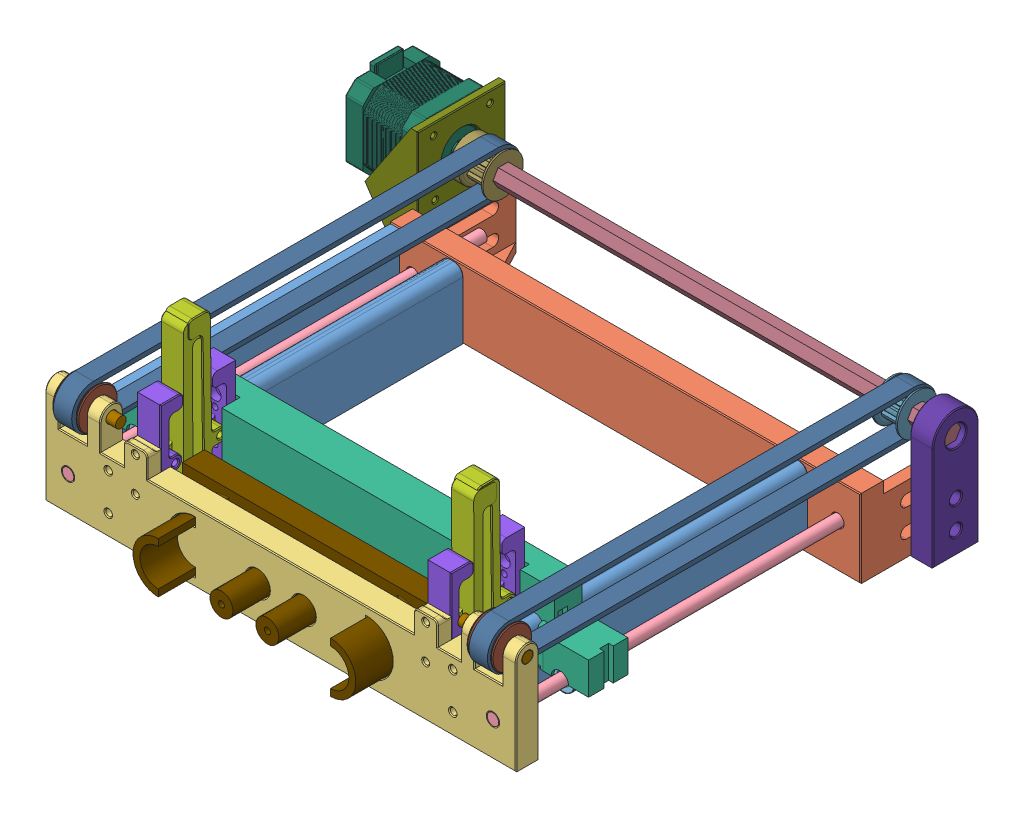
SolidWorks assembly Full Gantry Assembly COPY, configuration Default. Lengths in mm.
Overall size (316.36 107.99 274.71).
39 component instances, 19 part files, 30 mates.
Components (placement in the parent):
- Gantry Frame Assembly-1: Gantry Frame Assembly [Default] at (-22.7812 29.2709 55.0882) size (260.35 63.5 254)
  - Frame Side Walls-1: Frame Side Walls [Default] at (-11.2932 98.0952 84.9503) size (12.1 37.5 177.8)
  - Gantry Frame End Piece-1: Gantry Frame End Piece [Default] at (83.9568 98.3952 72.2503) size (260.35 43.18 63.5)
  - Gantry Frame Heating End Piece-1: Gantry Frame Heating End Piece [Default] at (83.9568 98.3952 262.7503) size (260.35 58.42 12.7)
  - Frame Side Walls-2: Frame Side Walls [Default] at (179.2068 98.0952 84.9503) size (12.1 37.5 177.8)
  - 0.25 Diam 9 inch long Linear Rod-1: 0.25 Diam 9 inch long Linear Rod [Default] at (201.4318 98.3952 46.8503) x (0.968537 -0.248869 0) z (0 0 1) size (6.35 6.35 228.6)
  - 0.25 Diam 9 inch long Linear Rod-2: 0.25 Diam 9 inch long Linear Rod [Default] at (-33.5182 98.3952 46.8503) x (0.995745 -0.092157 0) z (0 0 1) size (6.35 6.35 228.6)
- Gantry Subassembly-1: Gantry Subassembly [Default] at (-16.8456 119.8156 318.0932) size (266.7 99.55 38.74)
  - 60595K11_Fixed Alignment Linear Ball Bearing-1: 60595K11_Fixed Alignment Linear Ball Bearing [60595K11] at (-39.4539 7.8505 -35.6605) size (12.7 12.7 19.05)
  - Gantry Piece-1: Gantry Piece [Default] at (78.0211 25.6305 -35.6605) size (266.7 50.8 22.23)
  - 60595K11_Fixed Alignment Linear Ball Bearing-2: 60595K11_Fixed Alignment Linear Ball Bearing [60595K11] at (195.4961 7.8505 -35.6605) x (0.99266 0.120939 0) z (0 0 1) size (12.7 12.7 19.05)
  - Clip Assembly-1: Clip Assembly [Default] at (45.7541 -13.0009 -33.2659) x (0 0.02134 0.999772) z (-1 0 0) size (28.26 95.92 12.7)
    - Added Clip Piece-1: Added Clip Piece [Default] at (13.6312 56.6752 41.3294) x (0.999405 -0.034486 0) z (0 0 1) size (20.96 95.25 12.7)
    - Attatched Clip Piece-1: Attatched Clip Piece [Default] at (0.3891 41.1725 54.0294) x (-0.999772 0.02134 0) z (0 0 -1) size (12.7 63.5 12.7)
  - Clip Assembly-2: Clip Assembly [Default] at (205.6471 -13.0009 -33.2659) x (0 0.02134 0.999772) z (-1 0 0) size (28.26 95.92 12.7)
    - Added Clip Piece-1: Added Clip Piece [Default] at (13.6312 56.6752 41.3294) x (0.999405 -0.034486 0) z (0 0 1) size (20.96 95.25 12.7)
    - Attatched Clip Piece-1: Attatched Clip Piece [Default] at (0.3891 41.1725 54.0294) x (-0.999772 0.02134 0) z (0 0 -1) size (12.7 63.5 12.7)
- Clip Assembly-1: Clip Assembly [Default] at (93.7601 105.5448 319.8889) x (0 0.02134 -0.999772) z (1 0 0) size (27.33 95.65 12.7) (flexible)
  - Added Clip Piece-1: Added Clip Piece [Default] at (13.4006 56.7842 41.3294) x (0.999804 -0.019788 0) z (0 0 1) size (20.96 95.25 12.7)
  - Attatched Clip Piece-1: Attatched Clip Piece [Default] at (0.3891 41.1725 54.0294) x (-0.999772 0.02134 0) z (0 0 -1) size (12.7 63.5 12.7)
- Clip Assembly-2: Clip Assembly [Default] at (-66.7679 105.5448 319.8889) x (0 0.02134 -0.999772) z (1 0 0) size (27.36 95.66 12.7) (flexible)
  - Added Clip Piece-1: Added Clip Piece [Default] at (13.4085 56.7805 41.3294) x (0.999794 -0.020292 0) z (0 0 1) size (20.96 95.25 12.7)
  - Attatched Clip Piece-1: Attatched Clip Piece [Default] at (0.3891 41.1725 54.0294) x (-0.999772 0.02134 0) z (0 0 -1) size (12.7 63.5 12.7)
- Passive Pulley Axle-1: Passive Pulley Axle [Default] at (-68.9995 160.6862 324.1885) x (0 -0.395908 -0.91829) z (0 -0.91829 0.395908) size (5.85 35.56 5.85)
- Passive Pulley Axle-2: Passive Pulley Axle [Default] at (191.3505 160.6862 324.1885) x (0 -0.802318 -0.596897) z (0 0.596897 -0.802318) size (5.85 35.56 5.85)
- Pulley and Belt Assembly-1: Pulley and Belt Assembly [Default] at (-262.393 22.4987 259.1542) x (0 0 -1) z (1 0 0) size (254.91 31.32 266.45) (flexible)
  - 20 Inch Belt-1: 20 Inch Belt [Default] at (47.0039 138.1875 203.6424) size (248.21 24.13 10.16)
  - Belt Idler Pulley-1: Belt Idler Pulley [6495K744] at (-65.0343 138.1875 212.2657) x (0.999956 -0.009357 0) z (0 0 1) size (22.23 22.23 14.3)
  - Belt Idler Pulley Coupler-1: Belt Idler Pulley Coupler [6495K744] at (159.0421 138.1875 205.9411) x (0.5 0.866025 0) z (0 0 -1) size (22.23 22.23 19.13)
  - Hexshaft Motor Drive Axle-1: Hexshaft Motor Drive Axle [Default] at (159.2153 138.1875 463.5733) x (0.5 -0.866025 0) z (0.866025 0.5 0) size (11 254 9.53)
  - Belt Idler Pulley Hex Hole-1: Belt Idler Pulley Hex Hole [6495K744] at (159.2153 138.1875 441.1959) x (-0.5 -0.866025 0) z (0 0 1) size (22.23 22.23 14.3)
  - Belt Idler Pulley-2: Belt Idler Pulley [6495K744] at (-64.8611 138.1875 441.1959) x (0.643871 0.765134 0) z (0 0 1) size (22.23 22.23 14.3)
  - 20 Inch Belt-2: 20 Inch Belt [Default] at (47.1771 138.1875 443.4946) x (1 0 0) z (0 0 -1) size (248.21 24.13 10.16)
- Stepper Mount and Tensioner-1: Stepper Mount and Tensioner [Default] at (-96.2784 207.8478 159.2914) x (1 0 0) z (0 -0.924225 0.381849) size (61.75 74.03 91.46)
  - Stepper Motor-1: Stepper Motor [Default] at (4.7189 -72.7035 20.9904) x (0 -0.924225 -0.381849) z (1 0 0) size (42.5 46.5 61.75)
  - Stepper Motor Mount-2: Stepper Motor Mount [Default] at (27.2789 -72.7035 20.9904) x (-1 0 0) z (0 -0.924225 -0.381849) size (29.21 76.08 48.66)
- Opposite tensioner-1: Opposite tensioner [Default] at (191.3505 103.5362 112.6389) x (0 0 -1) z (1 0 0) size (25.4 69.85 12.7)
- Spring Board-2: Spring Board [Default] at (-11.2145 108.6162 299.6968) x (1 0 0) z (0 -1 0) size (144.78 50.8 38.1)
- Part4^Full Gantry Assembly COPY-1: Part4^Full Gantry Assembly COPY [Default] at (61.1755 127.6662 140.0385) size (5.08 42.18 177.8) (virtual)
Mates (geometry in assembly coordinates):
- Concentric1: concentric aligned: cylinder of Gantry Frame Assembly-1/0.25 Diam 9 inch long Linear Rod-2 through (-56.2995 127.6662 330.5385) axis (0 0 -1) radius 3.175; cylinder of Gantry Subassembly-1/60595K11_Fixed Alignment Linear Ball Bearing-1 through (-56.2995 127.6662 282.4327) axis (0 0 -1) radius 3.175
- Concentric2: concentric aligned: cylinder of Gantry Frame Assembly-1/0.25 Diam 9 inch long Linear Rod-1 through (178.6505 127.6662 330.5385) axis (0 0 -1) radius 3.175; cylinder of Gantry Subassembly-1/60595K11_Fixed Alignment Linear Ball Bearing-2 through (178.6505 127.6662 282.4327) axis (0 0 -1) radius 3.175
- Parallel1: parallel anti-aligned: plane of Gantry Frame Assembly-1/Frame Side Walls-2 through (150.3755 141.0362 317.8385) normal (-1 0 0); plane of Clip Assembly-1/Added Clip Piece-1 through (147.7895 118.7851 308.9051) normal (1 0 0)
- Concentric5: concentric aligned: cylinder of Gantry Frame Assembly-1/Gantry Frame Heating End Piece-1 through (141.4395 155.6062 330.5385) axis (0 0 -1) radius 1.7; cylinder of Clip Assembly-1/Attatched Clip Piece-1 through (141.4395 155.6062 338.1585) axis (0 0 -1) radius 1.7
- Parallel2: parallel anti-aligned: plane of Gantry Frame Assembly-1/Frame Side Walls-2 through (150.3755 141.0362 317.8385) normal (-1 0 0); plane of Clip Assembly-2/Added Clip Piece-1 through (-12.7385 118.7822 308.9192) normal (1 0 0)
- Concentric6: concentric aligned: cylinder of Gantry Frame Assembly-1/Gantry Frame Heating End Piece-1 through (-19.0885 155.6062 330.5385) axis (0 0 -1) radius 1.7; cylinder of Clip Assembly-2/Attatched Clip Piece-1 through (-19.0885 155.6062 338.1585) axis (0 0 -1) radius 1.7
- Concentric7: concentric anti-aligned: cylinder of Gantry Frame Assembly-1/Gantry Frame Heating End Piece-1 through (-134.0235 160.6862 324.1885) axis (1 0 0) radius 3.175; cylinder of Passive Pulley Axle-1 through (-33.4395 160.6862 324.1885) axis (-1 0 0) radius 2.925
- Coincident5: coincident aligned: plane of Gantry Frame Assembly-1/Gantry Frame Heating End Piece-1 through (-68.9995 146.7162 330.5385) normal (-1 0 0); plane of Passive Pulley Axle-1 through (-68.9995 160.6862 324.1885) normal (-1 0 0)
- Concentric10: concentric aligned: cylinder of Gantry Frame Assembly-1/Gantry Frame Heating End Piece-1 through (-134.0235 160.6862 324.1885) axis (1 0 0) radius 3.175; cylinder of Passive Pulley Axle-2 through (155.7905 160.6862 324.1885) axis (1 0 0) radius 2.925
- Coincident7: coincident aligned: plane of Gantry Frame Assembly-1/Gantry Frame Heating End Piece-1 through (191.3505 146.7162 330.5385) normal (1 0 0); plane of Passive Pulley Axle-2 through (191.3505 160.6862 324.1885) normal (1 0 0)
- Concentric11: concentric anti-aligned: cylinder of Passive Pulley Axle-1 through (-33.4395 160.6862 324.1885) axis (-1 0 0) radius 2.925; cylinder of Pulley and Belt Assembly-1/Belt Idler Pulley-1 through (-39.8149 160.6862 324.1885) axis (1 0 0) radius 3.175
- Coincident8: coincident anti-aligned: plane of Gantry Frame Assembly-1/Gantry Frame Heating End Piece-1 through (-46.1395 167.0362 330.5385) normal (-1 0 0); plane of Pulley and Belt Assembly-1/Belt Idler Pulley-1 through (-46.1395 157.5113 324.2182) normal (1 0 0)
- Parallel3: parallel aligned: plane of Gantry Subassembly-1/Gantry Piece-1 through (-46.7745 145.4462 272.9077) normal (0 1 0); plane of Pulley and Belt Assembly-1/20 Inch Belt-1 through (-48.5906 172.7512 324.1885) normal (0 1 0)
- Coincident10: coincident anti-aligned: plane of Gantry Frame Assembly-1/Gantry Frame Heating End Piece-1 through (168.4905 167.0362 330.5385) normal (1 0 0); plane of Pulley and Belt Assembly-1/Belt Idler Pulley-2 through (168.4905 153.5312 315.5127) normal (-1 0 0)
- Parallel9: parallel aligned: plane of Gantry Frame Assembly-1/Gantry Frame End Piece-1 through (61.1755 103.5362 127.3385) normal (0 -1 0); plane of Stepper Mount and Tensioner-1/Stepper Motor Mount-2 through (-72.8095 105.8113 121.9021) normal (0 -1 0)
- Slot1: slot aligned: cylinder of Stepper Mount and Tensioner-1/Stepper Motor Mount-2 through (-72.8095 130.8412 100.1121) axis (1 0 0) radius 3.175; plane of Gantry Frame Assembly-1/Gantry Frame End Piece-1 through (-113.4495 127.6662 89.2385) normal (0 1 0); cylinder of Gantry Frame Assembly-1/Gantry Frame End Piece-1 through (-113.4495 130.8412 114.6385) axis (1 0 0) radius 3.175
- Slot2: slot aligned: cylinder of Stepper Mount and Tensioner-1/Stepper Motor Mount-2 through (-72.8095 115.6012 100.1121) axis (1 0 0) radius 3.175; plane of Gantry Frame Assembly-1/Gantry Frame End Piece-1 through (-113.4495 112.4262 89.2385) normal (0 1 0); cylinder of Gantry Frame Assembly-1/Gantry Frame End Piece-1 through (-113.4495 115.6012 114.6385) axis (1 0 0) radius 3.175
- Coincident18: coincident anti-aligned: plane of Gantry Frame Assembly-1/Gantry Frame End Piece-1 through (-68.9995 146.7162 140.0385) normal (-1 0 0); plane of Stepper Mount and Tensioner-1/Stepper Motor Mount-2 through (-68.9995 160.6862 100.1121) normal (1 0 0)
- Coincident19: coincident anti-aligned: plane of Gantry Frame Assembly-1/Gantry Frame End Piece-1 through (191.3505 146.7162 140.0385) normal (1 0 0); plane of Opposite tensioner-1 through (191.3505 160.6862 99.9389) normal (-1 0 0)
- Slot3: slot aligned: plane of Gantry Frame Assembly-1/Gantry Frame End Piece-1 through (235.8005 127.6662 89.2385) normal (0 1 0); cylinder of Opposite tensioner-1 through (204.0505 130.8412 99.9389) axis (-1 0 0) radius 3.175; cylinder of Gantry Frame Assembly-1/Gantry Frame End Piece-1 through (235.8005 130.8412 89.2385) axis (-1 0 0) radius 3.175
- Slot4: slot aligned: plane of Gantry Frame Assembly-1/Gantry Frame End Piece-1 through (235.8005 112.4262 89.2385) normal (0 1 0); cylinder of Opposite tensioner-1 through (204.0505 115.6012 99.9389) axis (-1 0 0) radius 3.175; cylinder of Gantry Frame Assembly-1/Gantry Frame End Piece-1 through (235.8005 115.6012 89.2385) axis (-1 0 0) radius 3.175
- Concentric12: concentric: cylinder of Pulley and Belt Assembly-1/Belt Idler Pulley Coupler-1 through (-66.7643 160.6862 100.1121) axis (-1 0 0) radius 2.5; cylinder of Stepper Mount and Tensioner-1/Stepper Motor-1 through (-50.5595 160.6862 100.1121) axis (-1 0 0) radius 2.5
- Concentric15: concentric anti-aligned: cylinder of Pulley and Belt Assembly-1/Belt Idler Pulley Hex Hole-1 through (189.1153 160.6862 99.9389) axis (1 0 0) radius 11.1125; cylinder of Opposite tensioner-1 through (204.0505 160.6862 99.9389) axis (-1 0 0) radius 5.715
- Concentric16: concentric anti-aligned: cylinder of Gantry Frame Assembly-1/Gantry Frame Heating End Piece-1 through (48.4755 127.6662 317.8385) axis (0 0 1) radius 6.6; cylinder of Spring Board-2 through (48.4755 127.6662 350.4968) axis (0 0 -1) radius 6.35
- Concentric17: concentric anti-aligned: cylinder of Gantry Frame Assembly-1/Gantry Frame Heating End Piece-1 through (73.8755 127.6662 317.8385) axis (0 0 1) radius 6.6; cylinder of Spring Board-2 through (73.8755 127.6662 350.4968) axis (0 0 -1) radius 6.35
- Coincident21: coincident anti-aligned: plane of Gantry Frame Assembly-1/Gantry Frame Heating End Piece-1 through (145.5035 156.8762 322.9185) normal (0 0 -1); plane of Clip Assembly-1/Attatched Clip Piece-1 through (135.0895 178.4662 322.9185) normal (0 0 1)
- InPlace1: in place: plane of Gantry Frame Assembly-1/Gantry Frame End Piece-1 through (61.1755 127.6662 140.0385) normal (0 0 1); plane of ? through (0 0 140.0385) normal (0 0 1); moOrthogonalPlaneRef_w of Gantry Frame Assembly-1/Gantry Frame End Piece-1 through (61.1755 127.6662 140.0385) normal (0 0 1); plane of ? through (0 0 140.0385) normal (0 1 0); plane of Gantry Frame Assembly-1/Gantry Frame End Piece-1 through (61.1755 127.6662 140.0385) normal (0 0 1); plane of ? through (0 0 140.0385) normal (1 0 0); plane of Gantry Frame Assembly-1/Gantry Frame End Piece-1 through (61.1755 127.6662 140.0385) normal (0 0 1); unknown of Part4^Full Gantry Assembly COPY-1
- Coincident22: coincident aligned: plane of Gantry Frame Assembly-1/Gantry Frame End Piece-1; plane of Part4^Full Gantry Assembly COPY-1
- Coincident23: coincident aligned: moOrthogonalPlaneRef_w of Gantry Frame Assembly-1/Gantry Frame End Piece-1 through (61.1755 127.6662 140.0385) normal (0 1 0); plane of Part4^Full Gantry Assembly COPY-1 through (61.1755 127.6662 140.0385) normal (0 1 0)
- Coincident24: coincident anti-aligned: moOrthogonalPlaneRef_w of Gantry Frame Assembly-1/Gantry Frame End Piece-1 through (61.1755 127.6662 140.0385) normal (-1 0 0); plane of Part4^Full Gantry Assembly COPY-1 through (61.1755 127.6662 140.0385) normal (1 0 0)
